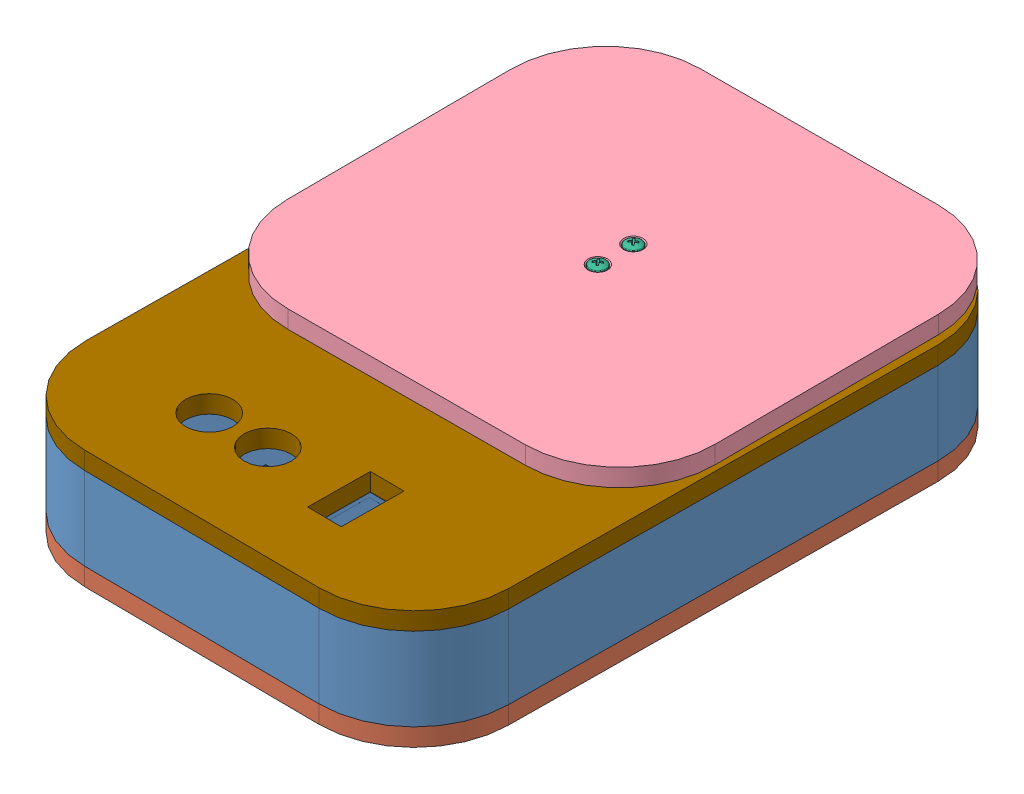
SolidWorks assembly Main, configuration Default. Lengths in mm.
Overall size (182.26 61.96 261.56).
18 component instances, 11 part files, 16 mates.
Components (placement in the parent):
- mail wall-1: mail wall [Default] at (468.1099 74.0645 -181.95) x (-0.999962 0 -0.008727) z (0.008727 0 -0.999962) size (180 35 260)
- bottom lid-2: bottom lid [Default] at (468.1099 31.5645 -181.95) x (0.999962 0 0.008727) z (-0.008727 0 0.999962) size (180 7.5 260)
- Loadcell-1kg-No Name.step-1: Loadcell-1kg-No Name.step [Default] at (468.4825 94.8439 -197.5959) x (0 0 1) z (-1 0 0) size (91.8 14.23 13.91)
- tray-1: tray [Default] at (468.6751 134.9439 -266.3463) x (0.999991 0 -0.00428) z (0.00428 0 0.999991) size (180 7.5 175)
- Part5-1: Part5 [Default] at origin size (12.6 12.5 27.5)
- pan cross head_am-1: pan cross head_am [B18.6.7M - M3.5 x 0.6 x 35 Type I Cross Recessed PHMS --35N] at (468.4825 128.4614 -232.8459) x (0 -1 0) z (-0.788636 0 0.61486) size (37.57 7 7)
- pan cross head_am-3: pan cross head_am [B18.6.7M - M3.5 x 0.6 x 35 Type I Cross Recessed PHMS --35N] at (468.4825 128.5554 -217.8459) x (0 -1 0) z (0.792721 0 -0.609585) size (37.57 7 7)
- Part1-1: Part1 [Default] at origin size (50 22.7 32.99)
- hex bolt_am-1: hex bolt_am [B18.2.3.5M - Hex bolt M5 x 0.8 x 35 --16N] at (468.8184 72.2139 -162.6607) x (0 1 0) z (0 0 1) size (38.58 9.24 8)
- hex bolt_am-2: hex bolt_am [B18.2.3.5M - Hex bolt M5 x 0.8 x 35 --16N] at (468.8184 72.2139 -177.7301) x (0 1 0) z (0 0 1) size (38.58 9.24 8)
- Top lid with second pcb-2: Top lid with second pcb [Default] at (567.0429 -14.7467 22.0801) x (-0.999962 0 -0.008727) z (0.008727 0 -0.999962) size (180 18.64 260)
  - top lid-1: top lid [Default] at (100.7096 131.3112 203.159) size (180 7.5 260)
  - second_pcb.step-1: second_pcb.step [Default] at (17.5816 118.1729 -168.5329) x (0 0 -1) z (0 1 0) size (33.15 95 11)
  - Part64-1: Part64 [Default] at origin size (95.93 5.6 34.46)
  - pan cross head_am-2: pan cross head_am [B18.6.7M - M4 x 0.7 x 10 Type I Cross Recessed PHMS --10C] at (61.2696 114.6615 128.1391) x (0 1 0) z (0.253418 0 0.967357) size (13.07 8 8)
  - pan cross head_am-3: pan cross head_am [B18.6.7M - M4 x 0.7 x 10 Type I Cross Recessed PHMS --10C] at (152.2016 114.6615 127.7581) x (0 1 0) z (-0.971066 0 -0.238809) size (13.07 8 8)
  - pan cross head_am-4: pan cross head_am [B18.6.7M - M4 x 0.7 x 10 Type I Cross Recessed PHMS --10C] at (152.2016 114.6615 98.6751) x (0 1 0) z (-0.342128 0 -0.939653) size (13.07 8 8)
  - pan cross head_am-5: pan cross head_am [B18.6.7M - M4 x 0.7 x 10 Type I Cross Recessed PHMS --10C] at (61.2696 114.6615 98.6751) x (0 1 0) z (-0.923859 0 -0.382733) size (13.07 8 8)
Mates (geometry in assembly coordinates):
- Coincident5: coincident anti-aligned: plane of Loadcell-1kg-No Name.step-1 through (468.4825 107.4439 -197.5959) normal (0 1 0); plane of Part5-1 through (0 107.4439 0) normal (0 -1 0)
- Coincident6: coincident anti-aligned: line of Loadcell-1kg-No Name.step-1 through (474.7825 107.4439 -237.5959) axis (-1 0 0); line of Part5-1 through (462.1825 107.4439 -237.5959) axis (1 0 0)
- Coincident8: coincident aligned: line of Loadcell-1kg-No Name.step-1 through (474.7825 107.4439 -157.5959) axis (0 0 -1); line of Part5-1 through (474.7825 107.4439 -210.0959) axis (0 0 -1)
- Concentric12: concentric aligned: cylinder of Part5-1 through (468.4825 127.4439 -232.8459) axis (0 1 0) radius 1.85; cylinder of pan cross head_am-1 through (468.4825 153.8614 -232.8459) axis (0 1 0) radius 1.75
- Coincident9: coincident aligned: cylinder of tray-1 through (468.4825 127.4439 -232.8459) axis (0 1 0) radius 1.85; circle of Part5-1
- Concentric15: concentric aligned: circle of tray-1; cylinder of pan cross head_am-3 through (468.4825 153.9554 -217.8459) axis (0 1 0) radius 1.75
- Concentric17: concentric aligned: cylinder of Part1-1 through (468.8184 72.1439 -162.6607) axis (0 -1 0) radius 2.65; cylinder of hex bolt_am-1 through (468.8184 72.2139 -162.6607) axis (0 -1 0) radius 2.5
- Concentric18: concentric aligned: cylinder of Part1-1 through (468.8184 72.1439 -177.7301) axis (0 -1 0) radius 2.65; cylinder of hex bolt_am-2 through (468.8184 72.2139 -177.7301) axis (0 -1 0) radius 2.5
- Coincident10: coincident anti-aligned: plane of Part1-1 through (471.4684 75.7939 -177.7301) normal (0 -1 0); plane of hex bolt_am-2 through (464.1996 75.7939 -177.7301) normal (0 1 0)
- Coincident11: coincident anti-aligned: plane of Part1-1 through (471.4684 75.7939 -162.6607) normal (0 -1 0); plane of hex bolt_am-1 through (464.1996 75.7939 -162.6607) normal (0 1 0)
- Coincident18: coincident anti-aligned: line of mail wall-1 through (516.9736 74.0645 -51.5186) axis (-0.999962 0 -0.008727); line of bottom lid-2 through (416.9774 74.0645 -52.3913) axis (0.999962 0 0.008727)
- Coincident19: coincident aligned: line of mail wall-1 through (557.3211 74.0645 -91.168) axis (0.008727 0 -0.999962); line of bottom lid-2 through (557.3211 74.0645 -91.168) axis (0.008727 0 -0.999962)
- Lock1: lock: unknown of mail wall-1; unknown of bottom lid-2
- Lock2: lock: unknown of bottom lid-2; unknown of Part1-1
- Coincident22: coincident aligned: line of mail wall-1 through (516.9736 109.0645 -51.5186) axis (-0.999962 0 -0.008727); line of Top lid with second pcb-2/top lid-1 through (516.9736 109.0645 -51.5186) axis (-0.999962 0 -0.008727)
- Coincident23: coincident aligned: line of mail wall-1 through (377.328 109.0645 -92.7388) axis (0.008727 0 -0.999962); line of Top lid with second pcb-2/top lid-1 through (377.328 109.0645 -92.7388) axis (0.008727 0 -0.999962)
